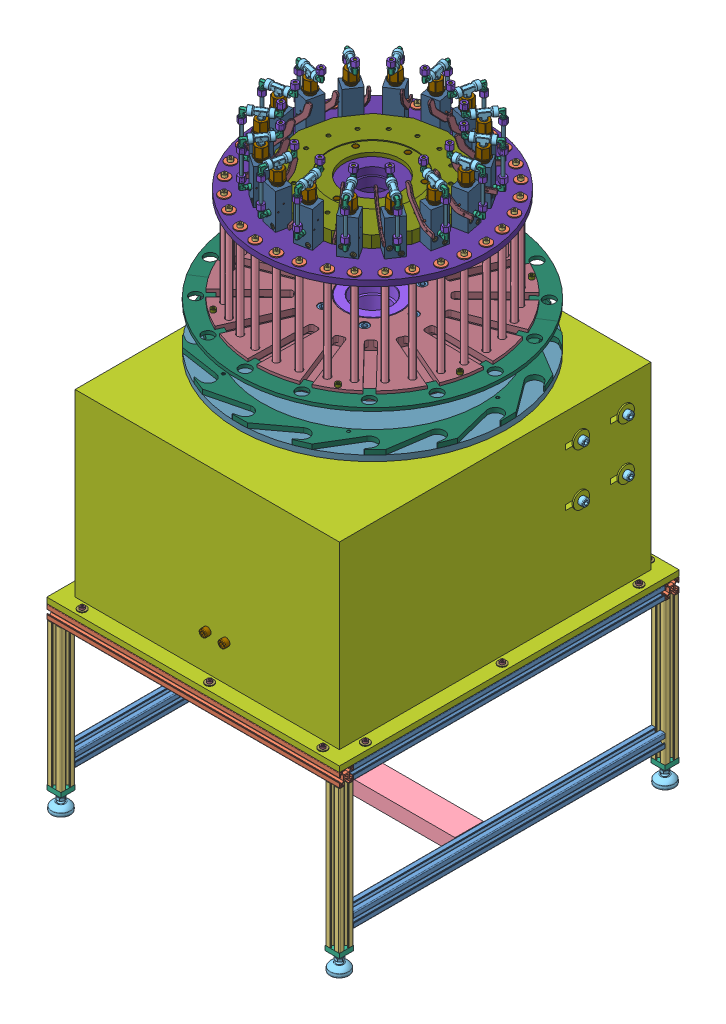
SolidWorks assembly Assieme_FINALE, configuration Default. Lengths in mm. (continued)
Components (placement in the parent): (continued)
- assieme parte rotante-1: assieme parte rotante [Default] at (-50.0904 623.9178 -607.5231) x (0 1 0) z (-0.804112 0 0.594478) size (749.63 778.63 778.63) (continued)
  - AssiemeValvola-4: AssiemeValvola [Default] at (515.3257 -108.3081 301.6234) x (0 0.745128 0.666921) z (0 0.666921 -0.745128) size (90.26 138.63 38) (continued)
    - Raccordo a L-3: Raccordo a L [Default] at (-30 -88.2824 0) x (0 1 0) z (0 0 1) size (28.34 25.51 14.01)
      - 1809_06_10_01-1: 1809_06_10_01 [Default] at origin size (22.49 23 10)
      - 1809_06_10_02-1: 1809_06_10_02 [Default] at origin size (6.5 8.5 8.5)
      - 1809_06_10_03-1: 1809_06_10_03 [Default] at origin size (11.02 15.01 14.01)
    - Spina_3x38-1: Spina_3x38 [Default] at (0 -68.2824 -21) x (-1 0 0) z (0 0 1) size (3 3 38)
    - Spina_3x38-2: Spina_3x38 [Default] at (-10 -80.2824 -21) x (0.996193 0.087174 0) z (0 0 1) size (3 3 38)
    - M5 40mm-3: M5 40mm [ISO 4762 M5 x 40 - 40N] at (-14.6 -108.7824 9) size (45 8.5 8.5)
    - M5 40mm-2: M5 40mm [ISO 4762 M5 x 40 - 40N] at (-14.6 -96.7824 -9) size (45 8.5 8.5)
    - LevaValvola-1: LevaValvola [Default] at (-24.507 -86.571 -17) x (0.996193 0.087174 0) z (0 0 1) size (77.55 60.2 4)
    - Tubo-1: Tubo [Default] at (-30 -15.9665 0) x (1 0 0) z (0 -1 0) size (6 6 56.4)
  - AssiemeValvola-5: AssiemeValvola [Default] at (515.3257 -142.0531 358.7289) x (0 0.943628 0.331007) z (0 0.331007 -0.943628) size (90.26 138.63 38)
    - RaccordoT-1: RaccordoT [Default] at origin size (43 29.75 16.5)
    - Raccordo a L-1: Raccordo a L [Default] at (-30 0 0) x (0 -1 0) z (0 0 -1) size (28.34 25.51 14.01)
      - 1809_06_10_01-1: 1809_06_10_01 [Default] at origin size (22.49 23 10)
      - 1809_06_10_02-1: 1809_06_10_02 [Default] at origin size (6.5 8.5 8.5)
      - 1809_06_10_03-1: 1809_06_10_03 [Default] at origin size (11.02 15.01 14.01)
    - Raccordo a L-2: Raccordo a L [Default] at (30 0 0) x (0 1 0) z (0 0 -1) size (28.34 25.51 14.01)
      - 1809_06_10_01-1: 1809_06_10_01 [Default] at origin size (22.49 23 10)
      - 1809_06_10_02-1: 1809_06_10_02 [Default] at origin size (6.5 8.5 8.5)
      - 1809_06_10_03-1: 1809_06_10_03 [Default] at origin size (11.02 15.01 14.01)
    - TappoChiusura-1: TappoChiusura [Default] at (0 -32 0) x (0 -1 0) z (0 0 1) size (38.28 26.74 26.74)
    - CorpoValvola-1: CorpoValvola [Default] at (-15 -115.2824 0) size (30 75 34)
    - Raccordo a L-3: Raccordo a L [Default] at (-30 -88.2824 0) x (0 1 0) z (0 0 1) size (28.34 25.51 14.01)
      - 1809_06_10_01-1: 1809_06_10_01 [Default] at origin size (22.49 23 10)
      - 1809_06_10_02-1: 1809_06_10_02 [Default] at origin size (6.5 8.5 8.5)
      - 1809_06_10_03-1: 1809_06_10_03 [Default] at origin size (11.02 15.01 14.01)
    - Spina_3x38-1: Spina_3x38 [Default] at (0 -68.2824 -21) x (-1 0 0) z (0 0 1) size (3 3 38)
    - Spina_3x38-2: Spina_3x38 [Default] at (-10 -80.2824 -21) x (0.996193 0.087174 0) z (0 0 1) size (3 3 38)
    - M5 40mm-3: M5 40mm [ISO 4762 M5 x 40 - 40N] at (-14.6 -108.7824 9) size (45 8.5 8.5)
    - M5 40mm-2: M5 40mm [ISO 4762 M5 x 40 - 40N] at (-14.6 -96.7824 -9) size (45 8.5 8.5)
    - LevaValvola-1: LevaValvola [Default] at (-24.507 -86.571 -17) x (0.996193 0.087174 0) z (0 0 1) size (77.55 60.2 4)
    - Tubo-1: Tubo [Default] at (-30 -15.9665 0) x (1 0 0) z (0 -1 0) size (6 6 56.4)
  - AssiemeValvola-6: AssiemeValvola [Default] at (515.3257 -151.3762 424.4011) x (0 0.99847 -0.055301) z (0 -0.055301 -0.99847) size (90.26 138.63 38)
    - RaccordoT-1: RaccordoT [Default] at origin size (43 29.75 16.5)
    - Raccordo a L-1: Raccordo a L [Default] at (-30 0 0) x (0 -1 0) z (0 0 -1) size (28.34 25.51 14.01)
      - 1809_06_10_01-1: 1809_06_10_01 [Default] at origin size (22.49 23 10)
      - 1809_06_10_02-1: 1809_06_10_02 [Default] at origin size (6.5 8.5 8.5)
      - 1809_06_10_03-1: 1809_06_10_03 [Default] at origin size (11.02 15.01 14.01)
    - Raccordo a L-2: Raccordo a L [Default] at (30 0 0) x (0 1 0) z (0 0 -1) size (28.34 25.51 14.01)
      - 1809_06_10_01-1: 1809_06_10_01 [Default] at origin size (22.49 23 10)
      - 1809_06_10_02-1: 1809_06_10_02 [Default] at origin size (6.5 8.5 8.5)
      - 1809_06_10_03-1: 1809_06_10_03 [Default] at origin size (11.02 15.01 14.01)
    - TappoChiusura-1: TappoChiusura [Default] at (0 -32 0) x (0 -1 0) z (0 0 1) size (38.28 26.74 26.74)
    - CorpoValvola-1: CorpoValvola [Default] at (-15 -115.2824 0) size (30 75 34)
    - Raccordo a L-3: Raccordo a L [Default] at (-30 -88.2824 0) x (0 1 0) z (0 0 1) size (28.34 25.51 14.01)
      - 1809_06_10_01-1: 1809_06_10_01 [Default] at origin size (22.49 23 10)
      - 1809_06_10_02-1: 1809_06_10_02 [Default] at origin size (6.5 8.5 8.5)
      - 1809_06_10_03-1: 1809_06_10_03 [Default] at origin size (11.02 15.01 14.01)
    - Spina_3x38-1: Spina_3x38 [Default] at (0 -68.2824 -21) x (-1 0 0) z (0 0 1) size (3 3 38)
    - Spina_3x38-2: Spina_3x38 [Default] at (-10 -80.2824 -21) x (0.996193 0.087174 0) z (0 0 1) size (3 3 38)
    - M5 40mm-3: M5 40mm [ISO 4762 M5 x 40 - 40N] at (-14.6 -108.7824 9) size (45 8.5 8.5)
    - M5 40mm-2: M5 40mm [ISO 4762 M5 x 40 - 40N] at (-14.6 -96.7824 -9) size (45 8.5 8.5)
    - LevaValvola-1: LevaValvola [Default] at (-24.507 -86.571 -17) x (0.996193 0.087174 0) z (0 0 1) size (77.55 60.2 4)
    - Tubo-1: Tubo [Default] at (-30 -15.9665 0) x (1 0 0) z (0 -1 0) size (6 6 56.4)
  - AssiemeValvola-7: AssiemeValvola [Default] at (515.3257 -134.8578 488.6421) x (0 0.901303 -0.433189) z (0 -0.433189 -0.901303) size (90.26 138.63 38)
    - RaccordoT-1: RaccordoT [Default] at origin size (43 29.75 16.5)
    - Raccordo a L-1: Raccordo a L [Default] at (-30 0 0) x (0 -1 0) z (0 0 -1) size (28.34 25.51 14.01)
      - 1809_06_10_01-1: 1809_06_10_01 [Default] at origin size (22.49 23 10)
      - 1809_06_10_02-1: 1809_06_10_02 [Default] at origin size (6.5 8.5 8.5)
      - 1809_06_10_03-1: 1809_06_10_03 [Default] at origin size (11.02 15.01 14.01)
    - Raccordo a L-2: Raccordo a L [Default] at (30 0 0) x (0 1 0) z (0 0 -1) size (28.34 25.51 14.01)
      - 1809_06_10_01-1: 1809_06_10_01 [Default] at origin size (22.49 23 10)
      - 1809_06_10_02-1: 1809_06_10_02 [Default] at origin size (6.5 8.5 8.5)
      - 1809_06_10_03-1: 1809_06_10_03 [Default] at origin size (11.02 15.01 14.01)
    - TappoChiusura-1: TappoChiusura [Default] at (0 -32 0) x (0 -1 0) z (0 0 1) size (38.28 26.74 26.74)
    - CorpoValvola-1: CorpoValvola [Default] at (-15 -115.2824 0) size (30 75 34)
    - Raccordo a L-3: Raccordo a L [Default] at (-30 -88.2824 0) x (0 1 0) z (0 0 1) size (28.34 25.51 14.01)
      - 1809_06_10_01-1: 1809_06_10_01 [Default] at origin size (22.49 23 10)
      - 1809_06_10_02-1: 1809_06_10_02 [Default] at origin size (6.5 8.5 8.5)
      - 1809_06_10_03-1: 1809_06_10_03 [Default] at origin size (11.02 15.01 14.01)
    - Spina_3x38-1: Spina_3x38 [Default] at (0 -68.2824 -21) x (-1 0 0) z (0 0 1) size (3 3 38)
    - Spina_3x38-2: Spina_3x38 [Default] at (-10 -80.2824 -21) x (0.996193 0.087174 0) z (0 0 1) size (3 3 38)
    - M5 40mm-3: M5 40mm [ISO 4762 M5 x 40 - 40N] at (-14.6 -108.7824 9) size (45 8.5 8.5)
    - M5 40mm-2: M5 40mm [ISO 4762 M5 x 40 - 40N] at (-14.6 -96.7824 -9) size (45 8.5 8.5)
    - LevaValvola-1: LevaValvola [Default] at (-24.507 -86.571 -17) x (0.996193 0.087174 0) z (0 0 1) size (77.55 60.2 4)
    - Tubo-1: Tubo [Default] at (-30 -15.9665 0) x (1 0 0) z (0 -1 0) size (6 6 56.4)
  - AssiemeValvola-8: AssiemeValvola [Default] at (515.3257 -95.0129 541.6718) x (0 0.666921 -0.745128) z (0 -0.745128 -0.666921) size (90.26 138.63 38)
    - RaccordoT-1: RaccordoT [Default] at origin size (43 29.75 16.5)
    - Raccordo a L-1: Raccordo a L [Default] at (-30 0 0) x (0 -1 0) z (0 0 -1) size (28.34 25.51 14.01)
      - 1809_06_10_01-1: 1809_06_10_01 [Default] at origin size (22.49 23 10)
      - 1809_06_10_02-1: 1809_06_10_02 [Default] at origin size (6.5 8.5 8.5)
      - 1809_06_10_03-1: 1809_06_10_03 [Default] at origin size (11.02 15.01 14.01)
    - Raccordo a L-2: Raccordo a L [Default] at (30 0 0) x (0 1 0) z (0 0 -1) size (28.34 25.51 14.01)
      - 1809_06_10_01-1: 1809_06_10_01 [Default] at origin size (22.49 23 10)
      - 1809_06_10_02-1: 1809_06_10_02 [Default] at origin size (6.5 8.5 8.5)
      - 1809_06_10_03-1: 1809_06_10_03 [Default] at origin size (11.02 15.01 14.01)
    - TappoChiusura-1: TappoChiusura [Default] at (0 -32 0) x (0 -1 0) z (0 0 1) size (38.28 26.74 26.74)
    - CorpoValvola-1: CorpoValvola [Default] at (-15 -115.2824 0) size (30 75 34)
    - Raccordo a L-3: Raccordo a L [Default] at (-30 -88.2824 0) x (0 1 0) z (0 0 1) size (28.34 25.51 14.01)
      - 1809_06_10_01-1: 1809_06_10_01 [Default] at origin size (22.49 23 10)
      - 1809_06_10_02-1: 1809_06_10_02 [Default] at origin size (6.5 8.5 8.5)
      - 1809_06_10_03-1: 1809_06_10_03 [Default] at origin size (11.02 15.01 14.01)
    - Spina_3x38-1: Spina_3x38 [Default] at (0 -68.2824 -21) x (-1 0 0) z (0 0 1) size (3 3 38)
    - Spina_3x38-2: Spina_3x38 [Default] at (-10 -80.2824 -21) x (0.996193 0.087174 0) z (0 0 1) size (3 3 38)
    - M5 40mm-3: M5 40mm [ISO 4762 M5 x 40 - 40N] at (-14.6 -108.7824 9) size (45 8.5 8.5)
    - M5 40mm-2: M5 40mm [ISO 4762 M5 x 40 - 40N] at (-14.6 -96.7824 -9) size (45 8.5 8.5)
    - LevaValvola-1: LevaValvola [Default] at (-24.507 -86.571 -17) x (0.996193 0.087174 0) z (0 0 1) size (77.55 60.2 4)
    - Tubo-1: Tubo [Default] at (-30 -15.9665 0) x (1 0 0) z (0 -1 0) size (6 6 56.4)
  - AssiemeValvola-9: AssiemeValvola [Default] at (515.3257 -37.9074 575.4168) x (0 0.331007 -0.943628) z (0 -0.943628 -0.331007) size (90.26 138.63 38)
    - RaccordoT-1: RaccordoT [Default] at origin size (43 29.75 16.5)
    - Raccordo a L-1: Raccordo a L [Default] at (-30 0 0) x (0 -1 0) z (0 0 -1) size (28.34 25.51 14.01)
      - 1809_06_10_01-1: 1809_06_10_01 [Default] at origin size (22.49 23 10)
      - 1809_06_10_02-1: 1809_06_10_02 [Default] at origin size (6.5 8.5 8.5)
      - 1809_06_10_03-1: 1809_06_10_03 [Default] at origin size (11.02 15.01 14.01)
    - Raccordo a L-2: Raccordo a L [Default] at (30 0 0) x (0 1 0) z (0 0 -1) size (28.34 25.51 14.01)
      - 1809_06_10_01-1: 1809_06_10_01 [Default] at origin size (22.49 23 10)
      - 1809_06_10_02-1: 1809_06_10_02 [Default] at origin size (6.5 8.5 8.5)
      - 1809_06_10_03-1: 1809_06_10_03 [Default] at origin size (11.02 15.01 14.01)
    - TappoChiusura-1: TappoChiusura [Default] at (0 -32 0) x (0 -1 0) z (0 0 1) size (38.28 26.74 26.74)
    - CorpoValvola-1: CorpoValvola [Default] at (-15 -115.2824 0) size (30 75 34)
    - Raccordo a L-3: Raccordo a L [Default] at (-30 -88.2824 0) x (0 1 0) z (0 0 1) size (28.34 25.51 14.01)
      - 1809_06_10_01-1: 1809_06_10_01 [Default] at origin size (22.49 23 10)
      - 1809_06_10_02-1: 1809_06_10_02 [Default] at origin size (6.5 8.5 8.5)
      - 1809_06_10_03-1: 1809_06_10_03 [Default] at origin size (11.02 15.01 14.01)
    - Spina_3x38-1: Spina_3x38 [Default] at (0 -68.2824 -21) x (-1 0 0) z (0 0 1) size (3 3 38)
    - Spina_3x38-2: Spina_3x38 [Default] at (-10 -80.2824 -21) x (0.996193 0.087174 0) z (0 0 1) size (3 3 38)
    - M5 40mm-3: M5 40mm [ISO 4762 M5 x 40 - 40N] at (-14.6 -108.7824 9) size (45 8.5 8.5)
    - M5 40mm-2: M5 40mm [ISO 4762 M5 x 40 - 40N] at (-14.6 -96.7824 -9) size (45 8.5 8.5)
    - LevaValvola-1: LevaValvola [Default] at (-24.507 -86.571 -17) x (0.996193 0.087174 0) z (0 0 1) size (77.55 60.2 4)
    - Tubo-1: Tubo [Default] at (-30 -15.9665 0) x (1 0 0) z (0 -1 0) size (6 6 56.4)
  - AssiemeValvola-10: AssiemeValvola [Default] at (515.3257 27.7648 584.7399) x (0 -0.055301 -0.99847) z (0 -0.99847 0.055301) size (90.26 138.63 38)
    - RaccordoT-1: RaccordoT [Default] at origin size (43 29.75 16.5)
    - Raccordo a L-1: Raccordo a L [Default] at (-30 0 0) x (0 -1 0) z (0 0 -1) size (28.34 25.51 14.01)
      - 1809_06_10_01-1: 1809_06_10_01 [Default] at origin size (22.49 23 10)
      - 1809_06_10_02-1: 1809_06_10_02 [Default] at origin size (6.5 8.5 8.5)
      - 1809_06_10_03-1: 1809_06_10_03 [Default] at origin size (11.02 15.01 14.01)
    - Raccordo a L-2: Raccordo a L [Default] at (30 0 0) x (0 1 0) z (0 0 -1) size (28.34 25.51 14.01)
      - 1809_06_10_01-1: 1809_06_10_01 [Default] at origin size (22.49 23 10)
      - 1809_06_10_02-1: 1809_06_10_02 [Default] at origin size (6.5 8.5 8.5)
      - 1809_06_10_03-1: 1809_06_10_03 [Default] at origin size (11.02 15.01 14.01)
    - TappoChiusura-1: TappoChiusura [Default] at (0 -32 0) x (0 -1 0) z (0 0 1) size (38.28 26.74 26.74)
    - CorpoValvola-1: CorpoValvola [Default] at (-15 -115.2824 0) size (30 75 34)
    - Raccordo a L-3: Raccordo a L [Default] at (-30 -88.2824 0) x (0 1 0) z (0 0 1) size (28.34 25.51 14.01)
      - 1809_06_10_01-1: 1809_06_10_01 [Default] at origin size (22.49 23 10)
      - 1809_06_10_02-1: 1809_06_10_02 [Default] at origin size (6.5 8.5 8.5)
      - 1809_06_10_03-1: 1809_06_10_03 [Default] at origin size (11.02 15.01 14.01)
    - Spina_3x38-1: Spina_3x38 [Default] at (0 -68.2824 -21) x (-1 0 0) z (0 0 1) size (3 3 38)
    - Spina_3x38-2: Spina_3x38 [Default] at (-10 -80.2824 -21) x (0.996193 0.087174 0) z (0 0 1) size (3 3 38)
    - M5 40mm-3: M5 40mm [ISO 4762 M5 x 40 - 40N] at (-14.6 -108.7824 9) size (45 8.5 8.5)
    - M5 40mm-2: M5 40mm [ISO 4762 M5 x 40 - 40N] at (-14.6 -96.7824 -9) size (45 8.5 8.5)
    - LevaValvola-1: LevaValvola [Default] at (-24.507 -86.571 -17) x (0.996193 0.087174 0) z (0 0 1) size (77.55 60.2 4)
    - Tubo-1: Tubo [Default] at (-30 -15.9665 0) x (1 0 0) z (0 -1 0) size (6 6 56.4)
  - AssiemeValvola-11: AssiemeValvola [Default] at (515.3257 92.0058 568.2215) x (0 -0.433189 -0.901303) z (0 -0.901303 0.433189) size (90.26 138.63 38)
    - RaccordoT-1: RaccordoT [Default] at origin size (43 29.75 16.5)
    - Raccordo a L-1: Raccordo a L [Default] at (-30 0 0) x (0 -1 0) z (0 0 -1) size (28.34 25.51 14.01)
      - 1809_06_10_01-1: 1809_06_10_01 [Default] at origin size (22.49 23 10)
      - 1809_06_10_02-1: 1809_06_10_02 [Default] at origin size (6.5 8.5 8.5)
      - 1809_06_10_03-1: 1809_06_10_03 [Default] at origin size (11.02 15.01 14.01)
    - Raccordo a L-2: Raccordo a L [Default] at (30 0 0) x (0 1 0) z (0 0 -1) size (28.34 25.51 14.01)
      - 1809_06_10_01-1: 1809_06_10_01 [Default] at origin size (22.49 23 10)
      - 1809_06_10_02-1: 1809_06_10_02 [Default] at origin size (6.5 8.5 8.5)
      - 1809_06_10_03-1: 1809_06_10_03 [Default] at origin size (11.02 15.01 14.01)
    - TappoChiusura-1: TappoChiusura [Default] at (0 -32 0) x (0 -1 0) z (0 0 1) size (38.28 26.74 26.74)
    - CorpoValvola-1: CorpoValvola [Default] at (-15 -115.2824 0) size (30 75 34)
    - Raccordo a L-3: Raccordo a L [Default] at (-30 -88.2824 0) x (0 1 0) z (0 0 1) size (28.34 25.51 14.01)
      - 1809_06_10_01-1: 1809_06_10_01 [Default] at origin size (22.49 23 10)
      - 1809_06_10_02-1: 1809_06_10_02 [Default] at origin size (6.5 8.5 8.5)
      - 1809_06_10_03-1: 1809_06_10_03 [Default] at origin size (11.02 15.01 14.01)
    - Spina_3x38-1: Spina_3x38 [Default] at (0 -68.2824 -21) x (-1 0 0) z (0 0 1) size (3 3 38)
    - Spina_3x38-2: Spina_3x38 [Default] at (-10 -80.2824 -21) x (0.996193 0.087174 0) z (0 0 1) size (3 3 38)
    - M5 40mm-3: M5 40mm [ISO 4762 M5 x 40 - 40N] at (-14.6 -108.7824 9) size (45 8.5 8.5)
    - M5 40mm-2: M5 40mm [ISO 4762 M5 x 40 - 40N] at (-14.6 -96.7824 -9) size (45 8.5 8.5)
    - LevaValvola-1: LevaValvola [Default] at (-24.507 -86.571 -17) x (0.996193 0.087174 0) z (0 0 1) size (77.55 60.2 4)
    - Tubo-1: Tubo [Default] at (-30 -15.9665 0) x (1 0 0) z (0 -1 0) size (6 6 56.4)
  - AssiemeValvola-12: AssiemeValvola [Default] at (515.3257 145.0355 528.3766) x (0 -0.745128 -0.666921) z (0 -0.666921 0.745128) size (90.26 138.63 38)
    - RaccordoT-1: RaccordoT [Default] at origin size (43 29.75 16.5)
    - Raccordo a L-1: Raccordo a L [Default] at (-30 0 0) x (0 -1 0) z (0 0 -1) size (28.34 25.51 14.01)
      - 1809_06_10_01-1: 1809_06_10_01 [Default] at origin size (22.49 23 10)
      - 1809_06_10_02-1: 1809_06_10_02 [Default] at origin size (6.5 8.5 8.5)
      - 1809_06_10_03-1: 1809_06_10_03 [Default] at origin size (11.02 15.01 14.01)
    - Raccordo a L-2: Raccordo a L [Default] at (30 0 0) x (0 1 0) z (0 0 -1) size (28.34 25.51 14.01)
      - 1809_06_10_01-1: 1809_06_10_01 [Default] at origin size (22.49 23 10)
      - 1809_06_10_02-1: 1809_06_10_02 [Default] at origin size (6.5 8.5 8.5)
      - 1809_06_10_03-1: 1809_06_10_03 [Default] at origin size (11.02 15.01 14.01)
    - TappoChiusura-1: TappoChiusura [Default] at (0 -32 0) x (0 -1 0) z (0 0 1) size (38.28 26.74 26.74)
    - CorpoValvola-1: CorpoValvola [Default] at (-15 -115.2824 0) size (30 75 34)
    - Raccordo a L-3: Raccordo a L [Default] at (-30 -88.2824 0) x (0 1 0) z (0 0 1) size (28.34 25.51 14.01)
      - 1809_06_10_01-1: 1809_06_10_01 [Default] at origin size (22.49 23 10)
      - 1809_06_10_02-1: 1809_06_10_02 [Default] at origin size (6.5 8.5 8.5)
      - 1809_06_10_03-1: 1809_06_10_03 [Default] at origin size (11.02 15.01 14.01)
    - Spina_3x38-1: Spina_3x38 [Default] at (0 -68.2824 -21) x (-1 0 0) z (0 0 1) size (3 3 38)
    - Spina_3x38-2: Spina_3x38 [Default] at (-10 -80.2824 -21) x (0.996193 0.087174 0) z (0 0 1) size (3 3 38)
    - M5 40mm-3: M5 40mm [ISO 4762 M5 x 40 - 40N] at (-14.6 -108.7824 9) size (45 8.5 8.5)
    - M5 40mm-2: M5 40mm [ISO 4762 M5 x 40 - 40N] at (-14.6 -96.7824 -9) size (45 8.5 8.5)
    - LevaValvola-1: LevaValvola [Default] at (-24.507 -86.571 -17) x (0.996193 0.087174 0) z (0 0 1) size (77.55 60.2 4)
    - Tubo-1: Tubo [Default] at (-30 -15.9665 0) x (1 0 0) z (0 -1 0) size (6 6 56.4)
  - AssiemeValvola-13: AssiemeValvola [Default] at (515.3257 178.7805 471.2711) x (0 -0.943628 -0.331007) z (0 -0.331007 0.943628) size (90.26 138.63 38)
    - RaccordoT-1: RaccordoT [Default] at origin size (43 29.75 16.5)
    - Raccordo a L-1: Raccordo a L [Default] at (-30 0 0) x (0 -1 0) z (0 0 -1) size (28.34 25.51 14.01)
      - 1809_06_10_01-1: 1809_06_10_01 [Default] at origin size (22.49 23 10)
      - 1809_06_10_02-1: 1809_06_10_02 [Default] at origin size (6.5 8.5 8.5)
      - 1809_06_10_03-1: 1809_06_10_03 [Default] at origin size (11.02 15.01 14.01)
    - Raccordo a L-2: Raccordo a L [Default] at (30 0 0) x (0 1 0) z (0 0 -1) size (28.34 25.51 14.01)
      - 1809_06_10_01-1: 1809_06_10_01 [Default] at origin size (22.49 23 10)
      - 1809_06_10_02-1: 1809_06_10_02 [Default] at origin size (6.5 8.5 8.5)
      - 1809_06_10_03-1: 1809_06_10_03 [Default] at origin size (11.02 15.01 14.01)
    - TappoChiusura-1: TappoChiusura [Default] at (0 -32 0) x (0 -1 0) z (0 0 1) size (38.28 26.74 26.74)
    - CorpoValvola-1: CorpoValvola [Default] at (-15 -115.2824 0) size (30 75 34)
    - Raccordo a L-3: Raccordo a L [Default] at (-30 -88.2824 0) x (0 1 0) z (0 0 1) size (28.34 25.51 14.01)
      - 1809_06_10_01-1: 1809_06_10_01 [Default] at origin size (22.49 23 10)
      - 1809_06_10_02-1: 1809_06_10_02 [Default] at origin size (6.5 8.5 8.5)
      - 1809_06_10_03-1: 1809_06_10_03 [Default] at origin size (11.02 15.01 14.01)
    - Spina_3x38-1: Spina_3x38 [Default] at (0 -68.2824 -21) x (-1 0 0) z (0 0 1) size (3 3 38)
    - Spina_3x38-2: Spina_3x38 [Default] at (-10 -80.2824 -21) x (0.996193 0.087174 0) z (0 0 1) size (3 3 38)
    - M5 40mm-3: M5 40mm [ISO 4762 M5 x 40 - 40N] at (-14.6 -108.7824 9) size (45 8.5 8.5)
    - M5 40mm-2: M5 40mm [ISO 4762 M5 x 40 - 40N] at (-14.6 -96.7824 -9) size (45 8.5 8.5)
    - LevaValvola-1: LevaValvola [Default] at (-24.507 -86.571 -17) x (0.996193 0.087174 0) z (0 0 1) size (77.55 60.2 4)
    - Tubo-1: Tubo [Default] at (-30 -15.9665 0) x (1 0 0) z (0 -1 0) size (6 6 56.4)
  - AssiemeValvola-14: AssiemeValvola [Default] at (515.3257 188.1036 405.5989) x (0 -0.99847 0.055301) z (0 0.055301 0.99847) size (90.26 138.63 38)
    - RaccordoT-1: RaccordoT [Default] at origin size (43 29.75 16.5)
    - Raccordo a L-1: Raccordo a L [Default] at (-30 0 0) x (0 -1 0) z (0 0 -1) size (28.34 25.51 14.01)
      - 1809_06_10_01-1: 1809_06_10_01 [Default] at origin size (22.49 23 10)
      - 1809_06_10_02-1: 1809_06_10_02 [Default] at origin size (6.5 8.5 8.5)
      - 1809_06_10_03-1: 1809_06_10_03 [Default] at origin size (11.02 15.01 14.01)
    - Raccordo a L-2: Raccordo a L [Default] at (30 0 0) x (0 1 0) z (0 0 -1) size (28.34 25.51 14.01)
      - 1809_06_10_01-1: 1809_06_10_01 [Default] at origin size (22.49 23 10)
      - 1809_06_10_02-1: 1809_06_10_02 [Default] at origin size (6.5 8.5 8.5)
      - 1809_06_10_03-1: 1809_06_10_03 [Default] at origin size (11.02 15.01 14.01)
    - TappoChiusura-1: TappoChiusura [Default] at (0 -32 0) x (0 -1 0) z (0 0 1) size (38.28 26.74 26.74)
    - CorpoValvola-1: CorpoValvola [Default] at (-15 -115.2824 0) size (30 75 34)
    - Raccordo a L-3: Raccordo a L [Default] at (-30 -88.2824 0) x (0 1 0) z (0 0 1) size (28.34 25.51 14.01)
      - 1809_06_10_01-1: 1809_06_10_01 [Default] at origin size (22.49 23 10)
      - 1809_06_10_02-1: 1809_06_10_02 [Default] at origin size (6.5 8.5 8.5)
      - 1809_06_10_03-1: 1809_06_10_03 [Default] at origin size (11.02 15.01 14.01)
    - Spina_3x38-1: Spina_3x38 [Default] at (0 -68.2824 -21) x (-1 0 0) z (0 0 1) size (3 3 38)
    - Spina_3x38-2: Spina_3x38 [Default] at (-10 -80.2824 -21) x (0.996193 0.087174 0) z (0 0 1) size (3 3 38)
    - M5 40mm-3: M5 40mm [ISO 4762 M5 x 40 - 40N] at (-14.6 -108.7824 9) size (45 8.5 8.5)
    - M5 40mm-2: M5 40mm [ISO 4762 M5 x 40 - 40N] at (-14.6 -96.7824 -9) size (45 8.5 8.5)
    - LevaValvola-1: LevaValvola [Default] at (-24.507 -86.571 -17) x (0.996193 0.087174 0) z (0 0 1) size (77.55 60.2 4)
    - Tubo-1: Tubo [Default] at (-30 -15.9665 0) x (1 0 0) z (0 -1 0) size (6 6 56.4)
  - AssiemeValvola-15: AssiemeValvola [Default] at (515.3257 171.5852 341.3579) x (0 -0.901303 0.433189) z (0 0.433189 0.901303) size (90.26 138.63 38)
    - RaccordoT-1: RaccordoT [Default] at origin size (43 29.75 16.5)
    - Raccordo a L-1: Raccordo a L [Default] at (-30 0 0) x (0 -1 0) z (0 0 -1) size (28.34 25.51 14.01)
      - 1809_06_10_01-1: 1809_06_10_01 [Default] at origin size (22.49 23 10)
      - 1809_06_10_02-1: 1809_06_10_02 [Default] at origin size (6.5 8.5 8.5)
      - 1809_06_10_03-1: 1809_06_10_03 [Default] at origin size (11.02 15.01 14.01)
    - Raccordo a L-2: Raccordo a L [Default] at (30 0 0) x (0 1 0) z (0 0 -1) size (28.34 25.51 14.01)
      - 1809_06_10_01-1: 1809_06_10_01 [Default] at origin size (22.49 23 10)
      - 1809_06_10_02-1: 1809_06_10_02 [Default] at origin size (6.5 8.5 8.5)
      - 1809_06_10_03-1: 1809_06_10_03 [Default] at origin size (11.02 15.01 14.01)
    - TappoChiusura-1: TappoChiusura [Default] at (0 -32 0) x (0 -1 0) z (0 0 1) size (38.28 26.74 26.74)
    - CorpoValvola-1: CorpoValvola [Default] at (-15 -115.2824 0) size (30 75 34)
    - Raccordo a L-3: Raccordo a L [Default] at (-30 -88.2824 0) x (0 1 0) z (0 0 1) size (28.34 25.51 14.01)
      - 1809_06_10_01-1: 1809_06_10_01 [Default] at origin size (22.49 23 10)
      - 1809_06_10_02-1: 1809_06_10_02 [Default] at origin size (6.5 8.5 8.5)
      - 1809_06_10_03-1: 1809_06_10_03 [Default] at origin size (11.02 15.01 14.01)
    - Spina_3x38-1: Spina_3x38 [Default] at (0 -68.2824 -21) x (-1 0 0) z (0 0 1) size (3 3 38)
    - Spina_3x38-2: Spina_3x38 [Default] at (-10 -80.2824 -21) x (0.996193 0.087174 0) z (0 0 1) size (3 3 38)
    - M5 40mm-3: M5 40mm [ISO 4762 M5 x 40 - 40N] at (-14.6 -108.7824 9) size (45 8.5 8.5)
    - M5 40mm-2: M5 40mm [ISO 4762 M5 x 40 - 40N] at (-14.6 -96.7824 -9) size (45 8.5 8.5)
    - LevaValvola-1: LevaValvola [Default] at (-24.507 -86.571 -17) x (0.996193 0.087174 0) z (0 0 1) size (77.55 60.2 4)
    - Tubo-1: Tubo [Default] at (-30 -15.9665 0) x (1 0 0) z (0 -1 0) size (6 6 56.4)
  - AssiemeValvola-16: AssiemeValvola [Default] at (515.3257 131.7403 288.3282) x (0 -0.666921 0.745128) z (0 0.745128 0.666921) size (90.26 138.63 38)
    - RaccordoT-1: RaccordoT [Default] at origin size (43 29.75 16.5)
    - Raccordo a L-1: Raccordo a L [Default] at (-30 0 0) x (0 -1 0) z (0 0 -1) size (28.34 25.51 14.01)
      - 1809_06_10_01-1: 1809_06_10_01 [Default] at origin size (22.49 23 10)
      - 1809_06_10_02-1: 1809_06_10_02 [Default] at origin size (6.5 8.5 8.5)
      - 1809_06_10_03-1: 1809_06_10_03 [Default] at origin size (11.02 15.01 14.01)
    - Raccordo a L-2: Raccordo a L [Default] at (30 0 0) x (0 1 0) z (0 0 -1) size (28.34 25.51 14.01)
      - 1809_06_10_01-1: 1809_06_10_01 [Default] at origin size (22.49 23 10)
      - 1809_06_10_02-1: 1809_06_10_02 [Default] at origin size (6.5 8.5 8.5)
      - 1809_06_10_03-1: 1809_06_10_03 [Default] at origin size (11.02 15.01 14.01)
    - TappoChiusura-1: TappoChiusura [Default] at (0 -32 0) x (0 -1 0) z (0 0 1) size (38.28 26.74 26.74)
    - CorpoValvola-1: CorpoValvola [Default] at (-15 -115.2824 0) size (30 75 34)
    - Raccordo a L-3: Raccordo a L [Default] at (-30 -88.2824 0) x (0 1 0) z (0 0 1) size (28.34 25.51 14.01)
      - 1809_06_10_01-1: 1809_06_10_01 [Default] at origin size (22.49 23 10)
      - 1809_06_10_02-1: 1809_06_10_02 [Default] at origin size (6.5 8.5 8.5)
      - 1809_06_10_03-1: 1809_06_10_03 [Default] at origin size (11.02 15.01 14.01)
    - Spina_3x38-1: Spina_3x38 [Default] at (0 -68.2824 -21) x (-1 0 0) z (0 0 1) size (3 3 38)
    - Spina_3x38-2: Spina_3x38 [Default] at (-10 -80.2824 -21) x (0.996193 0.087174 0) z (0 0 1) size (3 3 38)
    - M5 40mm-3: M5 40mm [ISO 4762 M5 x 40 - 40N] at (-14.6 -108.7824 9) size (45 8.5 8.5)
    - M5 40mm-2: M5 40mm [ISO 4762 M5 x 40 - 40N] at (-14.6 -96.7824 -9) size (45 8.5 8.5)
    - LevaValvola-1: LevaValvola [Default] at (-24.507 -86.571 -17) x (0.996193 0.087174 0) z (0 0 1) size (77.55 60.2 4)
    - Tubo-1: Tubo [Default] at (-30 -15.9665 0) x (1 0 0) z (0 -1 0) size (6 6 56.4)
  - Disco alimentazione guarnizione fi24.4-1: Disco alimentazione guarnizione fi24.4 [Default] at (198.0433 18.3637 415) x (0 0.065403 0.997859) z (-1 0 0) size (570 285 7.35)
  - Disco alimentazione guarnizione fi24.4-2: Disco alimentazione guarnizione fi24.4 [Default] at (198.0433 18.3637 415) x (0 -0.065403 -0.997859) z (-1 0 0) size (570 285 7.35)
  - m6 12mm-1: m6 12mm [ISO 4762 M6 x 12 - 12N] at (210.0433 200.6849 574.8914) x (-1 0 0) z (0 0.793353 -0.608761) size (18 10 10)
  - m6 12mm-7: m6 12mm [ISO 4762 M6 x 12 - 12N] at (210.0433 260.3445 399.1397) x (-1 0 0) z (0 0.793353 -0.608761) size (18 10 10)
  - m6 12mm-8: m6 12mm [ISO 4762 M6 x 12 - 12N] at (210.0433 96.3128 185.3694) x (-1 0 0) z (0 0.793353 -0.608761) size (18 10 10)
  - m6 12mm-9: m6 12mm [ISO 4762 M6 x 12 - 12N] at (210.0433 -59.5854 644.6306) x (-1 0 0) z (0 -0.793353 -0.608761) size (18 10 10)
  - m6 12mm-10: m6 12mm [ISO 4762 M6 x 12 - 12N] at (210.0433 -223.6171 430.8603) x (-1 0 0) z (0 -0.793353 -0.608761) size (18 10 10)
  - m6 12mm-11: m6 12mm [ISO 4762 M6 x 12 - 12N] at (210.0433 -163.9575 255.1086) x (-1 0 0) z (0 0.793353 -0.608761) size (18 10 10)
Mates (geometry in assembly coordinates):
- Parallelo2: parallel aligned: plane of SupportoBase_Totale-2 through (4.0127 -14.4529 -3.9361) normal (0 1 0)
- Perpendicolare1: perpendicular: plane of SupportoBase_Totale-2 through (4.0127 -14.4529 -3.9361) normal (0 1 0)
- Parallelo4: parallel aligned: plane of SupportoBase_Totale-2 through (4.0127 -14.4529 -3.9361) normal (0 0 1)
- Coincidente5: coincident anti-aligned: plane of SupportoBase_Totale-2/assieme_base-1/Supporto di Base per macchina-1 through (-154.7135 275.9611 -15.5811) normal (-1 0 0); plane of motoriduttore-1 through (-154.7135 275.9611 -1179.5811) normal (1 0 0)
- Coincidente6: coincident aligned: plane of SupportoBase_Totale-2/assieme_base-1/Supporto di Base per macchina-1 through (-154.7135 467.9611 -697.5811) normal (0 0 -1); plane of motoriduttore-1 through (-154.7135 463.6811 -697.5811) normal (0 0 -1)
- Tangente1: tangent anti-aligned: plane of SupportoBase_Totale-2/assieme_base-1/Supporto di Base per macchina-1 through (-93.2286 597.9611 -659.5811) normal (0 1 0); cylinder of motoriduttore-1 through (-154.7135 603.4611 -650.5811) axis (-1 0 0) radius 5.5
- Concentrico1: concentric anti-aligned: cylinder of motoriduttore-1 through (-267.2135 442.7547 -597.5811) axis (0 1 0) radius 15; cylinder of Assieme_Riduttore-1/AlberoRiduttore-1 through (-267.2135 379.4375 -597.5811) axis (0 -1 0) radius 12.5
- Coincidente9: coincident anti-aligned: plane of motoriduttore-1 through (-164.7135 602.1811 -1179.5811) normal (0 1 0); plane of Assieme_Riduttore-1/Rondella di fermo-2 through (-267.2135 602.1811 -597.5811) normal (0 -1 0)
- Coincidente12: coincident anti-aligned: plane of socket head cap screw_iso-1 through (-131.7135 606.5159 -562.9749) normal (-1 0 0); plane of plain washer xlarge grade c_iso-1 through (-131.7135 596.9697 -539.8693) normal (1 0 0)
- Concentrico4: concentric aligned: cylinder of socket head cap screw_iso-1 through (-89.9635 603.4611 -555.5811) axis (1 0 0) radius 5; cylinder of plain washer xlarge grade c_iso-1 through (-99.7885 603.4611 -555.5811) axis (1 0 0) radius 5.5
- Coincidente13: coincident anti-aligned: plane of socket head cap screw_iso-2 through (-131.7135 484.4611 -555.5811) normal (-1 0 0); plane of plain washer xlarge grade c_iso-2 through (-131.7135 475.4611 -555.5811) normal (1 0 0)
- Concentrico5: concentric aligned: cylinder of socket head cap screw_iso-2 through (-89.9635 492.4611 -555.5811) axis (1 0 0) radius 5; cylinder of plain washer xlarge grade c_iso-2 through (-99.7885 492.4611 -555.5811) axis (1 0 0) radius 5.5
- Coincidente14: coincident anti-aligned: plane of socket head cap screw_iso-3 through (-131.7135 595.4611 -650.5811) normal (-1 0 0); plane of plain washer xlarge grade c_iso-4 through (-131.7135 586.4611 -650.5811) normal (1 0 0)
- Concentrico6: concentric aligned: cylinder of socket head cap screw_iso-3 through (-89.9635 603.4611 -650.5811) axis (1 0 0) radius 5; cylinder of plain washer xlarge grade c_iso-4 through (-99.7885 603.4611 -650.5811) axis (1 0 0) radius 5.5
- Coincidente15: coincident anti-aligned: plane of socket head cap screw_iso-4 through (-131.7135 484.4611 -650.5811) normal (-1 0 0); plane of plain washer xlarge grade c_iso-3 through (-131.7135 475.4611 -650.5811) normal (1 0 0)
- Concentrico7: concentric aligned: cylinder of socket head cap screw_iso-4 through (-89.9635 492.4611 -650.5811) axis (1 0 0) radius 5; cylinder of plain washer xlarge grade c_iso-3 through (-99.7885 492.4611 -650.5811) axis (1 0 0) radius 5.5
- Concentrico8: concentric anti-aligned: cylinder of motoriduttore-1 through (-154.7135 603.4611 -650.5811) axis (-1 0 0) radius 5.5; cylinder of socket head cap screw_iso-3 through (-89.9635 603.4611 -650.5811) axis (1 0 0) radius 5
- Coincidente16: coincident anti-aligned: plane of SupportoBase_Totale-2/assieme_base-1/Supporto di Base per macchina-1 through (-134.7135 287.9611 -15.5811) normal (1 0 0); plane of plain washer xlarge grade c_iso-4 through (-134.7135 597.9611 -650.5811) normal (-1 0 0)
- Concentrico9: concentric anti-aligned: cylinder of motoriduttore-1 through (-154.7135 603.4611 -555.5811) axis (-1 0 0) radius 5.5; cylinder of socket head cap screw_iso-1 through (-89.9635 603.4611 -555.5811) axis (1 0 0) radius 5
- Coincidente17: coincident anti-aligned: plane of SupportoBase_Totale-2/assieme_base-1/Supporto di Base per macchina-1 through (-134.7135 287.9611 -15.5811) normal (1 0 0); plane of plain washer xlarge grade c_iso-1 through (-134.7135 601.3609 -550.4979) normal (-1 0 0)
- Coincidente18: coincident anti-aligned: plane of SupportoBase_Totale-2/assieme_base-1/Supporto di Base per macchina-1 through (-134.7135 287.9611 -15.5811) normal (1 0 0); plane of plain washer xlarge grade c_iso-3 through (-134.7135 486.9611 -650.5811) normal (-1 0 0)
- Concentrico10: concentric aligned: circle of motoriduttore-1; cylinder of socket head cap screw_iso-4 through (-89.9635 492.4611 -650.5811) axis (1 0 0) radius 5
- Coincidente19: coincident anti-aligned: plane of SupportoBase_Totale-2/assieme_base-1/Supporto di Base per macchina-1 through (-134.7135 287.9611 -15.5811) normal (1 0 0); plane of plain washer xlarge grade c_iso-2 through (-134.7135 486.9611 -555.5811) normal (-1 0 0)
- Concentrico11: concentric aligned: circle of motoriduttore-1; cylinder of socket head cap screw_iso-2 through (-89.9635 492.4611 -555.5811) axis (1 0 0) radius 5
- Concentrico12: concentric anti-aligned: cylinder of socket head cap screw_iso-4 through (-89.9635 492.4611 -650.5811) axis (1 0 0) radius 5; cylinder of hex nut style 2 gradeab_iso-3 through (-164.7135 492.4611 -650.5811) axis (-1 0 0) radius 4.25
- Coincidente20: coincident anti-aligned: plane of motoriduttore-1 through (-164.7135 275.9611 -1179.5811) normal (-1 0 0); plane of hex nut style 2 gradeab_iso-3 through (-164.7135 501.6987 -650.5811) normal (1 0 0)
- Concentrico13: concentric anti-aligned: cylinder of socket head cap screw_iso-3 through (-89.9635 603.4611 -650.5811) axis (1 0 0) radius 5; cylinder of hex nut style 2 gradeab_iso-1 through (-164.7135 603.4611 -650.5811) axis (-1 0 0) radius 4.25
- Coincidente21: coincident aligned: plane of motoriduttore-1 through (-164.7135 275.9611 -1179.5811) normal (-1 0 0); circle of hex nut style 2 gradeab_iso-1
- Concentrico14: concentric anti-aligned: cylinder of socket head cap screw_iso-1 through (-89.9635 603.4611 -555.5811) axis (1 0 0) radius 5; cylinder of hex nut style 2 gradeab_iso-2 through (-164.7135 603.4611 -555.5811) axis (-1 0 0) radius 4.25
- Coincidente22: coincident anti-aligned: plane of motoriduttore-1 through (-164.7135 275.9611 -1179.5811) normal (-1 0 0); plane of hex nut style 2 gradeab_iso-2 through (-164.7135 612.6987 -555.5811) normal (1 0 0)
- Concentrico15: concentric anti-aligned: cylinder of socket head cap screw_iso-2 through (-89.9635 492.4611 -555.5811) axis (1 0 0) radius 5; cylinder of hex nut style 2 gradeab_iso-4 through (-164.7135 492.4611 -555.5811) axis (-1 0 0) radius 4.25
- Coincidente23: coincident anti-aligned: plane of motoriduttore-1 through (-164.7135 275.9611 -1179.5811) normal (-1 0 0); plane of hex nut style 2 gradeab_iso-4 through (-164.7135 501.6987 -555.5811) normal (1 0 0)
- Concentrico161: concentric aligned: cylinder of SupportoBase_Totale-2/assieme_base-1/canotto di supporto-1 through (-394.7135 587.1745 -375.5811) axis (0 1 0) radius 119; cylinder of assieme parte fissa-1/dado M20-3 through (-394.7135 692.9236 -375.5811) axis (0 1 0) radius 10
- Coincidente241: coincident anti-aligned: plane of SupportoBase_Totale-2/assieme_base-1/canotto di supporto-1 through (-394.7135 698.9611 -375.5811) normal (0 1 0); plane of assieme parte fissa-1/dado M20-3 through (-409.2137 698.9611 -385.0544) normal (0 -1 0)
- Concentrico17: concentric aligned: cylinder of SupportoBase_Totale-2/assieme_base-1/canotto di supporto-1 through (-394.7135 587.1745 -375.5811) axis (0 1 0) radius 67.5; cylinder of assieme parte rotante-1/albero rotazione piatti-1 through (-394.7135 684.3308 -375.5811) axis (0 1 0) radius 49.75
- Coincidente25: coincident anti-aligned: plane of SupportoBase_Totale-2/assieme_base-1/canotto di supporto-1 through (-394.7135 673.9611 -375.5811) normal (0 1 0); plane of assieme parte rotante-1/SKF - 6020 - 20,DE,NC,20_68-2 through (-382.0178 673.9611 -309.2858) normal (0 -1 0)
